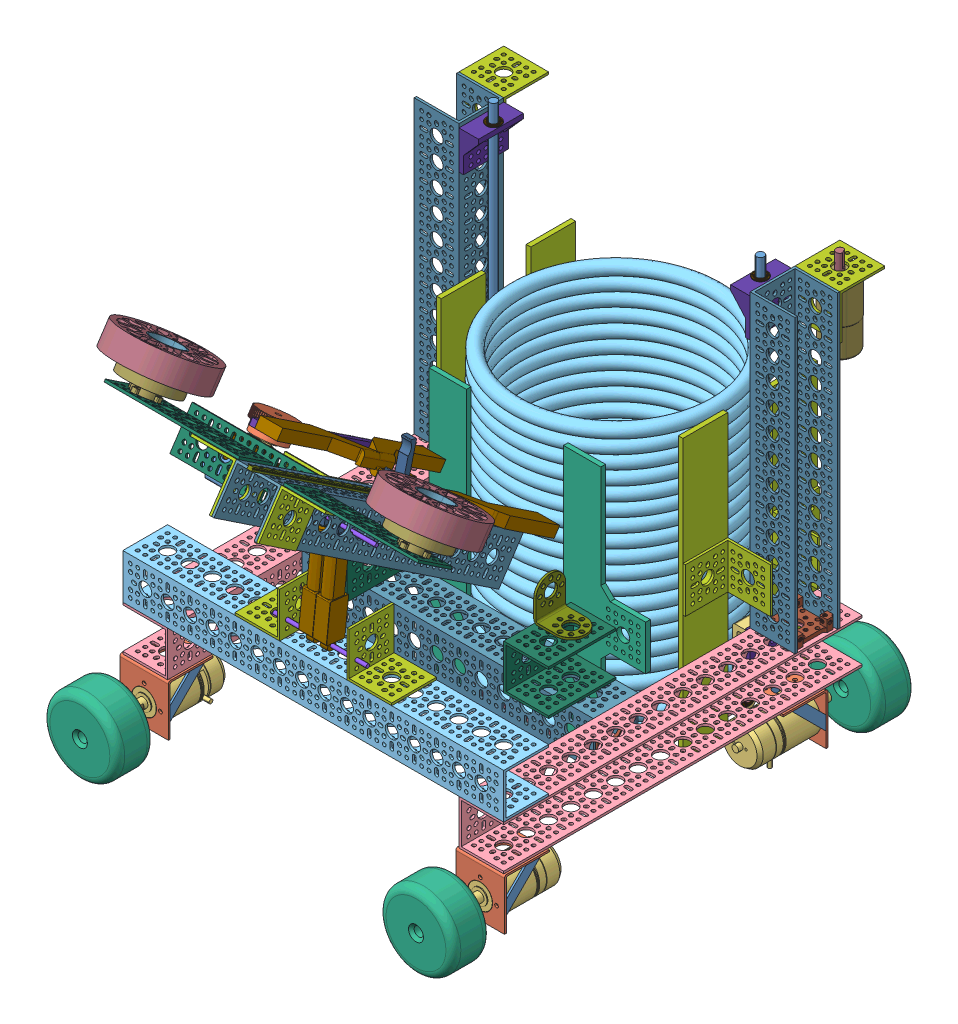
SolidWorks assembly 底座3.0, configuration 默认. Lengths in mm. (continued)
Mates (geometry in assembly coordinates): (continued)
- Concentric651: concentric anti-aligned: cylinder of 312mm-U型梁-7 through (105.3414 179.4201 525.5024) axis (0 1 0) radius 2; cone of 电机转向座-13 through (105.3414 186.9201 525.5024) axis (0 -1 0)
- Concentric652: concentric anti-aligned: cylinder of 312mm-U型梁-7 through (105.3414 181.4201 527.5024) axis (0 0 -1) radius 2; cone of 电机转向座-13 through (105.3414 181.4201 520.0024) axis (0 0 1)
- Concentric653: concentric anti-aligned: cylinder of 312mm-U型梁-7 through (105.3414 149.4201 527.5024) axis (0 0 -1) radius 2; cone of 电机转向座-13 through (105.3414 149.4201 520.0024) axis (0 0 1)
- Coincident318: coincident anti-aligned: plane of 384mm-U型梁-2 through (113.3414 189.4201 325.5024) normal (-1 0 0); plane of 电机转向座-13 through (113.3414 165.4201 541.5024) normal (1 0 0)
- Concentric654: concentric aligned: cylinder of 384mm-U型梁-2 through (123.3414 165.4201 541.5024) axis (-1 0 0) radius 7; cylinder of 电机转向座-13 through (113.3414 165.4201 541.5024) axis (-1 0 0) radius 7
- Concentric655: concentric aligned: cylinder of 384mm-U型梁-2 through (123.3414 156.9349 533.0171) axis (-1 0 0) radius 2; cylinder of 电机转向座-13 through (109.3414 156.9349 533.0171) axis (-1 0 0) radius 2
- Coincident323: coincident anti-aligned: plane of 312mm-U型梁-7 through (113.3414 189.4201 565.5024) normal (0 1 0); plane of 72mm-U型梁-5 through (89.3414 189.4201 589.5024) normal (0 -1 0)
- Coincident324: coincident anti-aligned: plane of 312mm-U型梁-7 through (113.3414 189.4201 565.5024) normal (0 1 0); plane of 72mm-U型梁-6 through (-174.6586 189.4201 589.5024) normal (0 -1 0)
- Concentric666: concentric aligned: cylinder of 72mm-U型梁-5 through (65.3414 227.4201 541.5024) axis (0 1 0) radius 7; cylinder of 圆角90°法兰-7 through (65.3414 237.4201 541.5024) axis (0 1 0) radius 7
- Coincident325: coincident anti-aligned: plane of 72mm-U型梁-5 through (89.3414 237.4201 589.5024) normal (0 1 0); plane of 圆角90°法兰-7 through (41.3414 237.4201 557.5024) normal (0 -1 0)
- Concentric667: concentric aligned: cylinder of 72mm-U型梁-5 through (54.0277 234.4201 541.5024) axis (0 1 0) radius 2; cylinder of 圆角90°法兰-7 through (54.0277 237.4201 541.5024) axis (0 1 0) radius 2.025
- Coincident326: coincident anti-aligned: plane of 72mm-U型梁-6 through (-174.6586 237.4201 589.5024) normal (0 1 0); plane of 圆角90°法兰-8 through (-126.6586 237.4201 525.5024) normal (0 -1 0)
- Concentric673: concentric anti-aligned: circle of 电动推杆2-1; cylinder of 升降轴-2 through (5.3414 358.1283 689.4197) axis (-1 0 0) radius 2
- Concentric674: concentric anti-aligned: circle of 电动推杆2-2; cylinder of 升降轴-2 through (5.3414 358.1283 689.4197) axis (-1 0 0) radius 2
- Coincident329: coincident anti-aligned: plane of 384mm-U型梁-1 through (-246.6586 189.4201 325.5024) normal (0 1 0); plane of 电机转向座-12 through (-222.6586 189.4201 373.5024) normal (0 -1 0)
- Concentric678: concentric aligned: cylinder of 轴承座-1 through (100.3414 497.4201 373.5024) axis (0 -1 0) radius 7; cylinder of 8-14轴承-7 through (100.3414 497.4201 373.5024) axis (0 -1 0) radius 7
- Coincident330: coincident anti-aligned: plane of 轴承座-1 through (113.3414 497.4201 397.5024) normal (0 1 0); plane of 8-14轴承-7 through (100.3414 497.4201 373.5024) normal (0 -1 0)
- Coincident331: coincident anti-aligned: plane of 384mm-U型梁-2 through (113.3414 189.4201 325.5024) normal (-1 0 0); plane of 轴承座-2 through (113.3414 145.4201 397.5024) normal (1 0 0)
- Concentric679: concentric anti-aligned: cylinder of 384mm-U型梁-2 through (123.3414 181.4201 389.5024) axis (-1 0 0) radius 2; cylinder of 轴承座-2 through (95.3414 181.4201 389.5024) axis (1 0 0) radius 2.05
- Concentric680: concentric anti-aligned: cylinder of 384mm-U型梁-2 through (123.3414 181.4201 357.5024) axis (-1 0 0) radius 2; cylinder of 轴承座-2 through (95.3414 181.4201 357.5024) axis (1 0 0) radius 2.05
- Concentric681: concentric anti-aligned: cylinder of 轴承座-2 through (100.3414 145.4201 373.5024) axis (0 1 0) radius 7; cylinder of 8-14轴承-8 through (100.3414 150.4201 373.5024) axis (0 -1 0) radius 7
- Coincident332: coincident anti-aligned: plane of 轴承座-2 through (113.3414 150.4201 349.5024) normal (0 1 0); plane of 8-14轴承-8 through (100.3414 150.4201 373.5024) normal (0 -1 0)
- Concentric682: concentric anti-aligned: cylinder of 8-14轴承-8 through (100.3414 146.4201 373.5024) axis (0 1 0) radius 4; cylinder of 螺纹杆-3 through (100.3414 517.4201 373.5024) axis (0 -1 0) radius 4
- Distance15: distance = 20 mm aligned: plane of 螺纹杆-3 through (100.3414 517.4201 373.5024) normal (0 1 0); plane of 轴承座-1 through (113.3414 497.4201 397.5024) normal (0 1 0)
- Concentric684: concentric aligned: cylinder of 螺纹杆-3 through (100.3414 517.4201 373.5024) axis (0 -1 0) radius 4; cylinder of 切边螺纹滑块-1 through (100.3414 178.1581 373.5024) axis (0 -1 0) radius 3.35
- Concentric687: concentric anti-aligned: cylinder of 384mm-U型梁-1 through (-208.6586 181.4201 389.5024) axis (1 0 0) radius 2; cylinder of 轴承座-4 through (-180.6586 181.4201 389.5024) axis (-1 0 0) radius 2.05
- Concentric688: concentric anti-aligned: cylinder of 384mm-U型梁-1 through (-208.6586 181.4201 357.5024) axis (1 0 0) radius 2; cylinder of 轴承座-4 through (-180.6586 181.4201 357.5024) axis (-1 0 0) radius 2.05
- Coincident334: coincident anti-aligned: plane of 384mm-U型梁-1 through (-198.6586 141.4201 325.5024) normal (1 0 0); plane of 轴承座-4 through (-198.6586 145.4201 349.5024) normal (-1 0 0)
- Concentric689: concentric aligned: cylinder of 轴承座-3 through (-185.6586 497.4201 373.5024) axis (0 -1 0) radius 7; cylinder of 8-14轴承-9 through (-185.6586 497.4201 373.5024) axis (0 -1 0) radius 7
- Coincident335: coincident anti-aligned: plane of 轴承座-3 through (-198.6586 497.4201 349.5024) normal (0 1 0); plane of 8-14轴承-9 through (-185.6586 497.4201 373.5024) normal (0 -1 0)
- Concentric690: concentric anti-aligned: cylinder of 轴承座-4 through (-185.6586 145.4201 373.5024) axis (0 1 0) radius 7; cylinder of 8-14轴承-10 through (-185.6586 150.4201 373.5024) axis (0 -1 0) radius 7
- Coincident336: coincident anti-aligned: plane of 轴承座-4 through (-198.6586 150.4201 397.5024) normal (0 1 0); plane of 8-14轴承-10 through (-185.6586 150.4201 373.5024) normal (0 -1 0)
- Concentric691: concentric anti-aligned: cylinder of 8-14轴承-9 through (-185.6586 493.4201 373.5024) axis (0 1 0) radius 4; cylinder of 螺纹杆-4 through (-185.6586 517.4201 373.5024) axis (0 -1 0) radius 4
- Coincident337: coincident aligned: plane of 螺纹杆-3 through (100.3414 517.4201 373.5024) normal (0 1 0); plane of 螺纹杆-4 through (-185.6586 517.4201 373.5024) normal (0 1 0)
- Concentric692: concentric aligned: cylinder of 螺纹杆-4 through (-185.6586 517.4201 373.5024) axis (0 -1 0) radius 4; cylinder of 切边螺纹滑块-2 through (-185.6586 178.1581 373.5024) axis (0 -1 0) radius 3.35
- Coincident338: coincident aligned: plane of 切边螺纹滑块-1 through (100.3414 168.1581 373.5024) normal (0 1 0); plane of 切边螺纹滑块-2 through (-185.6586 168.1581 373.5024) normal (0 1 0)
- Concentric693: concentric anti-aligned: cylinder of 切边螺纹滑块-1 through (100.3414 163.1581 373.5024) axis (0 1 0) radius 5.1; cylinder of 转换块-1 through (100.3414 173.1581 373.5024) axis (0 -1 0) radius 5.5
- Concentric694: concentric aligned: cylinder of 切边螺纹滑块-1 through (100.3414 168.1581 365.5024) axis (0 -1 0) radius 1.75; cylinder of 转换块-1 through (100.3414 173.1581 365.5024) axis (0 -1 0) radius 1.75
- Coincident339: coincident anti-aligned: plane of 切边螺纹滑块-1 through (100.3414 168.1581 373.5024) normal (0 1 0); plane of 转换块-1 through (100.3414 168.1581 373.5024) normal (0 -1 0)
- Concentric695: concentric anti-aligned: cylinder of 切边螺纹滑块-2 through (-185.6586 163.1581 373.5024) axis (0 1 0) radius 5.1; cylinder of 转换块-2 through (-185.6586 173.1581 373.5024) axis (0 -1 0) radius 5.5
- Concentric696: concentric aligned: cylinder of 切边螺纹滑块-2 through (-185.6586 168.1581 365.5024) axis (0 -1 0) radius 1.75; cylinder of 转换块-2 through (-185.6586 173.1581 365.5024) axis (0 -1 0) radius 1.75
- Coincident340: coincident anti-aligned: plane of 切边螺纹滑块-2 through (-185.6586 168.1581 373.5024) normal (0 1 0); plane of 转换块-2 through (-185.6586 168.1581 373.5024) normal (0 -1 0)
- Concentric697: concentric aligned: cylinder of 384mm-U型梁-2 through (121.3414 179.4201 365.5024) axis (0 1 0) radius 2; cylinder of 电机转向座-9 through (121.3414 193.4201 365.5024) axis (0 1 0) radius 2
- Concentric698: concentric anti-aligned: cone of 电机转向座-9 through (121.3414 197.4201 352.0024) axis (0 0 1); cylinder of 312mm-U型梁-8 through (121.3414 197.4201 359.5024) axis (0 0 -1) radius 2
- Concentric699: concentric anti-aligned: cone of 电机转向座-9 through (153.3414 197.4201 352.0024) axis (0 0 1); cylinder of 312mm-U型梁-8 through (153.3414 197.4201 359.5024) axis (0 0 -1) radius 2
- Concentric700: concentric anti-aligned: cone of 电机转向座-9 through (116.1914 197.4201 357.5024) axis (1 0 0); cylinder of 312mm-U型梁-8 through (123.3414 197.4201 357.5024) axis (-1 0 0) radius 2
- Concentric701: concentric anti-aligned: cone of 电机转向座-9 through (116.1914 197.4201 389.5024) axis (1 0 0); cylinder of 312mm-U型梁-8 through (123.3414 197.4201 389.5024) axis (-1 0 0) radius 2
- Coincident341: coincident anti-aligned: plane of 轴承座-1 through (113.3414 497.4201 349.5024) normal (1 0 0); plane of 312mm-U型梁-8 through (113.3414 189.4201 349.5024) normal (-1 0 0)
- Concentric704: concentric anti-aligned: cylinder of 48x48-L形支架-17 through (153.3414 493.4201 339.5024) axis (0 0 1) radius 2; cylinder of 312mm-U型梁-8 through (153.3414 493.4201 359.5024) axis (0 0 -1) radius 2
- Concentric705: concentric anti-aligned: cylinder of 48x48-L形支架-17 through (121.3414 493.4201 339.5024) axis (0 0 1) radius 2; cylinder of 312mm-U型梁-8 through (121.3414 493.4201 359.5024) axis (0 0 -1) radius 2
- Coincident342: coincident anti-aligned: plane of 48x48-L形支架-17 through (113.3414 501.4201 349.5024) normal (0 0 1); plane of 312mm-U型梁-8 through (161.3414 189.4201 349.5024) normal (0 0 -1)
- Concentric706: concentric anti-aligned: cylinder of 轴承座-1 through (95.3414 477.4201 357.5024) axis (1 0 0) radius 2.05; cylinder of 312mm-U型梁-8 through (123.3414 477.4201 357.5024) axis (-1 0 0) radius 2
- Concentric707: concentric anti-aligned: cylinder of 轴承座-1 through (95.3414 477.4201 389.5024) axis (1 0 0) radius 2.05; cylinder of 312mm-U型梁-8 through (123.3414 477.4201 389.5024) axis (-1 0 0) radius 2
- Concentric708: concentric aligned: cylinder of 384mm-U型梁-1 through (-206.6586 179.4201 365.5024) axis (0 1 0) radius 2; cylinder of 电机转向座-12 through (-206.6586 193.4201 365.5024) axis (0 1 0) radius 2
- Concentric709: concentric anti-aligned: cone of 电机转向座-12 through (-238.6586 197.4201 352.0024) axis (0 0 1); cylinder of 312mm-U型梁-9 through (-238.6586 197.4201 359.5024) axis (0 0 -1) radius 2
- Concentric710: concentric anti-aligned: cone of 电机转向座-12 through (-206.6586 197.4201 352.0024) axis (0 0 1); cylinder of 312mm-U型梁-9 through (-206.6586 197.4201 359.5024) axis (0 0 -1) radius 2
- Concentric711: concentric anti-aligned: cone of 电机转向座-12 through (-201.1586 197.4201 357.5024) axis (-1 0 0); cylinder of 312mm-U型梁-9 through (-208.6586 197.4201 357.5024) axis (1 0 0) radius 2
- Concentric712: concentric anti-aligned: cone of 电机转向座-12 through (-201.1586 197.4201 389.5024) axis (-1 0 0); cylinder of 312mm-U型梁-9 through (-208.6586 197.4201 389.5024) axis (1 0 0) radius 2
- Concentric713: concentric anti-aligned: cylinder of 48x48-L形支架-18 through (-206.6586 493.4201 339.5024) axis (0 0 1) radius 2; cylinder of 312mm-U型梁-9 through (-206.6586 493.4201 359.5024) axis (0 0 -1) radius 2
- Concentric714: concentric anti-aligned: cylinder of 48x48-L形支架-18 through (-238.6586 493.4201 339.5024) axis (0 0 1) radius 2; cylinder of 312mm-U型梁-9 through (-238.6586 493.4201 359.5024) axis (0 0 -1) radius 2
- Coincident343: coincident anti-aligned: plane of 48x48-L形支架-18 through (-246.6586 501.4201 349.5024) normal (0 0 1); plane of 312mm-U型梁-9 through (-246.6586 189.4201 349.5024) normal (0 0 -1)
- Concentric715: concentric anti-aligned: cylinder of 轴承座-3 through (-180.6586 477.4201 357.5024) axis (-1 0 0) radius 2.05; cylinder of 312mm-U型梁-9 through (-208.6586 477.4201 357.5024) axis (1 0 0) radius 2
- Concentric716: concentric anti-aligned: cylinder of 轴承座-3 through (-180.6586 477.4201 389.5024) axis (-1 0 0) radius 2.05; cylinder of 312mm-U型梁-9 through (-208.6586 477.4201 389.5024) axis (1 0 0) radius 2
- Coincident344: coincident anti-aligned: plane of 轴承座-3 through (-198.6586 497.4201 397.5024) normal (-1 0 0); plane of 312mm-U型梁-9 through (-198.6586 189.4201 397.5024) normal (1 0 0)
- Parallel5: parallel aligned: plane of 转换块-1 through (82.3414 173.1581 361.5024) normal (-1 0 0); plane of 312mm-U型梁-8 through (113.3414 189.4201 349.5024) normal (-1 0 0)
- Parallel6: parallel aligned: plane of 转换块-2 through (-167.6586 173.1581 385.5024) normal (1 0 0); plane of 312mm-U型梁-9 through (-198.6586 189.4201 397.5024) normal (1 0 0)
- Concentric717: concentric aligned: cylinder of 转换块-1 through (142.3414 100.1581 373.5024) axis (-1 0 0) radius 7; cylinder of 8-14轴承-11 through (87.3414 100.1581 373.5024) axis (-1 0 0) radius 7
- Coincident345: coincident anti-aligned: plane of 转换块-1 through (87.3414 88.1581 361.5024) normal (1 0 0); plane of 8-14轴承-11 through (87.3414 100.1581 373.5024) normal (-1 0 0)
- Concentric718: concentric aligned: cylinder of 转换块-2 through (-227.6586 100.1581 373.5024) axis (1 0 0) radius 7; cylinder of 8-14轴承-12 through (-172.6586 100.1581 373.5024) axis (1 0 0) radius 7
- Coincident346: coincident anti-aligned: plane of 转换块-2 through (-172.6586 88.1581 385.5024) normal (-1 0 0); plane of 8-14轴承-12 through (-172.6586 100.1581 373.5024) normal (1 0 0)
- Concentric719: concentric aligned: cylinder of 8-14轴承-11 through (83.3414 100.1581 373.5024) axis (1 0 0) radius 4; cylinder of 铲板-1 through (-164.6586 100.1581 373.5024) axis (1 0 0) radius 6
- Coincident347: coincident anti-aligned: plane of 8-14轴承-11 through (83.3414 100.1581 373.5024) normal (-1 0 0); plane of 铲板-1 through (83.3414 100.1581 373.5024) normal (1 0 0)
- Concentric720: concentric aligned: cylinder of 72mm-U型梁-6 through (-150.6586 227.4201 541.5024) axis (0 1 0) radius 7; cylinder of 圆角90°法兰-8 through (-150.6586 237.4201 541.5024) axis (0 1 0) radius 7
- Concentric728: concentric aligned: cylinder of 72mm-U型梁-6 through (-150.6586 234.4201 530.1887) axis (0 1 0) radius 2; cylinder of 圆角90°法兰-8 through (-150.6586 237.4201 530.1887) axis (0 1 0) radius 2.025
- Coincident356: coincident anti-aligned: plane of 312mm-U型梁-9 through (-246.6586 189.4201 397.5024) normal (0 0 1); plane of 48x48-L形支架-22 through (-174.6586 213.4201 397.5024) normal (0 0 -1)
- Concentric742: concentric anti-aligned: cylinder of 312mm-U型梁-9 through (-206.6586 253.4201 387.5024) axis (0 0 1) radius 2; cylinder of 48x48-L形支架-22 through (-206.6586 253.4201 407.5024) axis (0 0 -1) radius 2
- Concentric743: concentric anti-aligned: cylinder of 312mm-U型梁-9 through (-214.6586 253.4201 387.5024) axis (0 0 1) radius 2; cylinder of 48x48-L形支架-22 through (-214.6586 253.4201 407.5024) axis (0 0 -1) radius 2
- Coincident357: coincident anti-aligned: plane of 312mm-U型梁-9 through (-246.6586 189.4201 349.5024) normal (0 0 -1); plane of 48x48-L形支架-23 through (-174.6586 261.4201 349.5024) normal (0 0 1)
- Concentric744: concentric anti-aligned: cylinder of 312mm-U型梁-9 through (-206.6586 253.4201 359.5024) axis (0 0 -1) radius 2; cylinder of 48x48-L形支架-23 through (-206.6586 253.4201 339.5024) axis (0 0 1) radius 2
- Concentric745: concentric anti-aligned: cylinder of 312mm-U型梁-9 through (-214.6586 253.4201 359.5024) axis (0 0 -1) radius 2; cylinder of 48x48-L形支架-23 through (-214.6586 253.4201 339.5024) axis (0 0 1) radius 2
- Concentric746: concentric anti-aligned: cylinder of 48x48-L形支架-23 through (-184.6586 237.4201 325.5024) axis (1 0 0) radius 7; cylinder of 侧挡板-1 through (-169.6586 237.4201 325.5024) axis (-1 0 0) radius 7
- Coincident358: coincident anti-aligned: plane of 48x48-L形支架-23 through (-174.6586 261.4201 301.5024) normal (1 0 0); plane of 侧挡板-1 through (-174.6586 77.4201 301.5024) normal (-1 0 0)
- Concentric747: concentric anti-aligned: cylinder of 48x48-L形支架-23 through (-184.6586 253.4201 341.5024) axis (1 0 0) radius 2; cylinder of 侧挡板-1 through (-169.6586 253.4201 341.5024) axis (-1 0 0) radius 2
- Concentric748: concentric anti-aligned: cylinder of 48x48-L形支架-22 through (-184.6586 237.4201 421.5024) axis (1 0 0) radius 7; cylinder of 侧挡板-2 through (-169.6586 237.4201 421.5024) axis (-1 0 0) radius 7
- Concentric749: concentric anti-aligned: cylinder of 48x48-L形支架-22 through (-184.6586 253.4201 437.5024) axis (1 0 0) radius 2; cylinder of 侧挡板-2 through (-169.6586 253.4201 437.5024) axis (-1 0 0) radius 2
- Coincident359: coincident anti-aligned: plane of 48x48-L形支架-22 through (-174.6586 213.4201 445.5024) normal (1 0 0); plane of 侧挡板-2 through (-174.6586 77.4201 397.5024) normal (-1 0 0)
- Coincident360: coincident anti-aligned: plane of 312mm-U型梁-8 through (161.3414 189.4201 349.5024) normal (0 0 -1); plane of 48x48-L形支架-24 through (137.3414 261.4201 349.5024) normal (0 0 1)
- Concentric750: concentric anti-aligned: cylinder of 312mm-U型梁-8 through (121.3414 253.4201 359.5024) axis (0 0 -1) radius 2; cylinder of 48x48-L形支架-24 through (121.3414 253.4201 339.5024) axis (0 0 1) radius 2
- Concentric751: concentric anti-aligned: cylinder of 312mm-U型梁-8 through (129.3414 253.4201 359.5024) axis (0 0 -1) radius 2; cylinder of 48x48-L形支架-24 through (129.3414 253.4201 339.5024) axis (0 0 1) radius 2
- Concentric752: concentric aligned: cylinder of 侧挡板-3 through (89.3414 237.4201 325.5024) axis (-1 0 0) radius 7; cylinder of 48x48-L形支架-24 through (99.3414 237.4201 325.5024) axis (-1 0 0) radius 7
- Coincident361: coincident anti-aligned: plane of 侧挡板-3 through (89.3414 77.4201 301.5024) normal (1 0 0); plane of 48x48-L形支架-24 through (89.3414 261.4201 349.5024) normal (-1 0 0)
- Concentric753: concentric aligned: cylinder of 侧挡板-3 through (89.3414 253.4201 309.5024) axis (-1 0 0) radius 2; cylinder of 48x48-L形支架-24 through (99.3414 253.4201 309.5024) axis (-1 0 0) radius 2
- Coincident362: coincident anti-aligned: plane of 312mm-U型梁-8 through (161.3414 189.4201 397.5024) normal (0 0 1); plane of 48x48-L形支架-25 through (89.3414 261.4201 397.5024) normal (0 0 -1)
- Concentric754: concentric anti-aligned: cylinder of 312mm-U型梁-8 through (121.3414 253.4201 387.5024) axis (0 0 1) radius 2; cylinder of 48x48-L形支架-25 through (121.3414 253.4201 407.5024) axis (0 0 -1) radius 2
- Concentric755: concentric anti-aligned: cylinder of 312mm-U型梁-8 through (129.3414 253.4201 387.5024) axis (0 0 1) radius 2; cylinder of 48x48-L形支架-25 through (129.3414 253.4201 407.5024) axis (0 0 -1) radius 2
- Concentric756: concentric aligned: cylinder of 侧挡板-4 through (89.3414 237.4201 421.5024) axis (-1 0 0) radius 7; cylinder of 48x48-L形支架-25 through (99.3414 237.4201 421.5024) axis (-1 0 0) radius 7
- Coincident363: coincident anti-aligned: plane of 侧挡板-4 through (89.3414 77.4201 397.5024) normal (1 0 0); plane of 48x48-L形支架-25 through (89.3414 261.4201 445.5024) normal (-1 0 0)
- Concentric757: concentric aligned: cylinder of 侧挡板-4 through (89.3414 253.4201 437.5024) axis (-1 0 0) radius 2; cylinder of 48x48-L形支架-25 through (99.3414 253.4201 437.5024) axis (-1 0 0) radius 2
- 同心2: concentric aligned: circle of 圆角90°法兰-8; circle of 312mm-U型梁-10
- 距离2: distance = 60 mm anti-aligned: plane of 312mm-U型梁-10 through (-66.6586 401.3085 794.3883) normal (-1 0 0); plane of 圆角90°法兰-8 through (-126.6586 237.4201 525.5024) normal (1 0 0)
- 同心9: concentric anti-aligned: circle of 312mm-U型梁-10; circle of 滑轨9-1
- 重合17: coincident anti-aligned: plane of 312mm-U型梁-10 through (-66.6586 441.2359 767.7462) normal (0 0.831822 -0.555042); plane of 滑轨9-1 through (-40.1586 271.5672 513.4695) normal (0 -0.831822 0.555042)
- 平行4: parallel aligned: plane of 312mm-U型梁-10 through (-21.1586 439.1564 769.1339) normal (-1 0 0); plane of 滑轨9-1 through (-45.1586 271.5672 513.4695) normal (-1 0 0)
- 重合19: coincident anti-aligned: plane of 蜘蛛钩子-1/滑块1-1 through (-40.1586 335.1761 602.1319) normal (0 -0.831822 0.555042); plane of 滑轨9-1 through (-45.1586 274.645 511.4159) normal (0 0.831822 -0.555042)
- 重合20: coincident: line of 蜘蛛钩子-1/滑块1-1 through (-44.6586 342.8091 616.2736) axis (-0.707107 -0.588187 0.392474); plane of 滑轨9-1 through (-44.6586 273.3972 512.2485) normal (-0.707107 0.588187 -0.392474)
- 重合21: coincident anti-aligned: plane of 蜘蛛钩子-1/滑块座1-1 through (-115.6586 311.2353 689.2916) normal (-1 0 0); plane of 齿条(1)-1 through (-115.6586 355.6063 610.1389) normal (1 0 0)
- 重合22: coincident aligned: plane of 蜘蛛钩子-1/滑块座1-1 through (-97.6586 375.7779 646.2249) normal (0 -0.831822 0.555042); plane of 齿条(1)-1 through (-123.1586 289.073 516.2832) normal (0 -0.831822 0.555042)
- 重合23: coincident aligned: plane of 蜘蛛钩子-1/滑块座1-1 through (-115.6586 403.6958 704.2795) normal (0 0.555042 0.831822); plane of 齿条(1)-1 through (-115.6586 408.2709 701.2268) normal (0 0.555042 0.831822)
- 重合30: coincident anti-aligned: plane of 齿轮(5.23)-1 through (-143.7715 366.6942 656.9339) normal (0 -0.831822 0.555042); plane of 舵盘(5.23-1 through (-143.7715 366.6942 656.9339) normal (0 0.831822 -0.555042)
- 重合31: coincident aligned: plane of 齿条(1)-1 through (-123.1586 294.4799 512.6754) normal (0 0.831822 -0.555042); plane of 齿轮(5.23)-1 through (-143.7715 383.3306 645.833) normal (0 0.831822 -0.555042)
- 同心16: concentric anti-aligned: circle of 312mm-U型梁-10; circle of 48x48-L形支架-27
- 重合34: coincident anti-aligned: plane of 312mm-U型梁-10 through (-66.6586 401.3085 794.3883) normal (-1 0 0); plane of 48x48-L形支架-27 through (-66.6586 347.9889 628.0001) normal (1 0 0)
- 同心17: concentric anti-aligned: cylinder of 312mm-U型梁-7 through (-166.6586 179.4201 557.5024) axis (0 1 0) radius 2; circle of 72mm-U型梁-6
- 同心19: concentric anti-aligned: circle of 312mm-U型梁-7; circle of 72mm-U型梁-5
- 同心20: concentric anti-aligned: circle of 圆角90°法兰-7; circle of 312mm-U型梁-10
- 同心5: concentric anti-aligned: circle of 发射法兰1-1; circle of 发射无刷电机-1
- 重合4: coincident anti-aligned: circle of 发射法兰1-1; plane of 发射无刷电机-1 through (-186.6586 458.3921 738.8671) normal (0 0.831822 -0.555042)
- 同心21: concentric anti-aligned: circle of 发射法兰1-1; circle of 摩擦轮-1/摩擦轮.STEP-1/3613-0014-0096 Core.STEP-1
- 重合5: coincident anti-aligned: plane of 发射法兰1-1 through (-186.6586 457.2783 728.1895) normal (0 0.831822 -0.555042); plane of 摩擦轮-1/摩擦轮.STEP-1/3613-0014-0096 Core.STEP-1 through (-186.6586 457.2783 728.1895) normal (0 -0.831822 0.555042)
- 同心22: concentric anti-aligned: circle of 发射无刷电机-1; circle of 5孔平板-1
- 重合3: coincident anti-aligned: plane of 发射无刷电机-1 through (-186.6586 429.9945 746.3949) normal (0 -0.831822 0.555042); plane of 5孔平板-1 through (-66.6586 418.0611 728.5107) normal (0 0.831822 -0.555042)
- 同心1: concentric aligned: unknown of 5孔平板-1; unknown of 48x48-L形支架-28
- 平行1: parallel aligned: plane of 5孔平板-1 through (-210.6586 435.9453 716.5773) normal (-1 0 0); plane of 48x48-L形支架-28 through (-114.6586 439.1564 769.1339) normal (-1 0 0)
- 同心23: concentric anti-aligned: circle of 312mm-U型梁-10; circle of 48x48-L形支架-28
- 重合35: coincident aligned: plane of 312mm-U型梁-10 through (-42.6586 439.1564 769.1339) normal (0 0.555042 0.831822); plane of 48x48-L形支架-28 through (-69.1586 421.2722 781.0673) normal (0 0.555042 0.831822)
- 重合36: coincident anti-aligned: plane of 312mm-U型梁-10 through (-66.6586 401.3085 794.3883) normal (-1 0 0); plane of 48x48-L形支架-28 through (-66.6586 441.2359 767.7462) normal (1 0 0)
- 同心24: concentric anti-aligned: circle of 发射法兰1-2; circle of 发射无刷电机-2
- 重合37: coincident anti-aligned: circle of 发射法兰1-2; plane of 发射无刷电机-2 through (101.3414 447.8463 723.0624) normal (0 0.831822 -0.555042)
- 同心6: concentric anti-aligned: circle of 发射法兰1-2; circle of 摩擦轮-2/摩擦轮.STEP-1/3613-0014-0096 Core.STEP-1
- 重合38: coincident anti-aligned: plane of 发射法兰1-2 through (101.3414 457.2783 728.1895) normal (0 0.831822 -0.555042); plane of 摩擦轮-2/摩擦轮.STEP-1/3613-0014-0096 Core.STEP-1 through (101.3414 457.2783 728.1895) normal (0 -0.831822 0.555042)
- 同心25: concentric anti-aligned: circle of 发射无刷电机-2; circle of 5孔平板-2
- 重合39: coincident anti-aligned: plane of 发射无刷电机-2 through (101.3414 429.9945 746.3949) normal (0 -0.831822 0.555042); plane of 5孔平板-2 through (-18.6586 441.9279 764.2791) normal (0 0.831822 -0.555042)
- 同心26: concentric aligned: unknown of 5孔平板-2; unknown of 48x48-L形支架-29
- 平行8: parallel aligned: plane of 5孔平板-2 through (125.3414 459.8121 752.3457) normal (1 0 0); plane of 48x48-L形支架-29 through (29.3414 412.5144 729.2064) normal (1 0 0)
- 同心27: concentric aligned: circle of 312mm-U型梁-10; circle of 48x48-L形支架-29
- 重合40: coincident aligned: plane of 312mm-U型梁-10 through (-42.6586 439.1564 769.1339) normal (0 0.555042 0.831822); plane of 48x48-L形支架-29 through (-16.1586 421.2722 781.0673) normal (0 0.555042 0.831822)
- 重合41: coincident anti-aligned: plane of 312mm-U型梁-10 through (-18.6586 401.3085 794.3883) normal (1 0 0); plane of 48x48-L形支架-29 through (-18.6586 414.5939 727.8188) normal (-1 0 0)
- 同心28: concentric aligned: circle of 舵机-1; circle of 多功能舵机支架(1)-1
- 重合2: coincident anti-aligned: plane of 舵机-1 through (-179.2715 356.9383 673.6621) normal (0 -0.831822 0.555042); plane of 多功能舵机支架(1)-1 through (-153.6215 359.7413 677.8628) normal (0 0.831822 -0.555042)
- 同心29: concentric anti-aligned: circle of 舵机-1; circle of 齿轮(5.23)-1
- 同心30: concentric anti-aligned: circle of 舵机-1; circle of 舵盘(5.23-1
- 重合42: coincident anti-aligned: plane of 舵机-1 through (-143.7715 362.951 659.4316) normal (0 0.831822 -0.555042); plane of 舵盘(5.23-1 through (-143.7715 362.951 659.4316) normal (0 -0.831822 0.555042)
- 平行9: parallel aligned: plane of 48x48-L形支架-28 through (-69.1586 421.2722 781.0673) normal (0 0.555042 0.831822); plane of 多功能舵机支架(1)-1 through (-182.6215 359.7413 677.8628) normal (0 0.555042 0.831822)
- 平行12: parallel anti-aligned: plane of 舵机-1 through (-179.2715 360.0168 673.4112) normal (0 0.555042 0.831822); plane of 多功能舵机支架(1)-1 through (-174.1215 332.4288 693.683) normal (0 -0.555042 -0.831822)
- 重合53: coincident anti-aligned: plane of 5孔平板-1 through (-66.6586 441.2359 767.7462) normal (0 -0.831822 0.555042); plane of 48x48-L形支架-28 through (-114.6586 441.2359 767.7462) normal (0 0.831822 -0.555042)
- 重合54: coincident anti-aligned: plane of 5孔平板-2 through (-18.6586 414.5939 727.8188) normal (0 -0.831822 0.555042); plane of 48x48-L形支架-29 through (29.3414 414.5939 727.8188) normal (0 0.831822 -0.555042)
- 平行13: parallel aligned: plane of 312mm-U型梁-10 through (-42.6586 439.1564 769.1339) normal (0 0.555042 0.831822); plane of 48x48-L形支架-27 through (-66.6586 374.6309 667.9276) normal (0 0.555042 0.831822)
- 同心38: concentric aligned: circle of 48x48-L形支架-27; circle of 5孔平板-3
- 重合57: coincident anti-aligned: plane of 48x48-L形支架-27 through (-66.6586 374.6309 667.9276) normal (0 0.555042 0.831822); plane of 5孔平板-3 through (-66.6586 334.7034 694.5696) normal (0 -0.555042 -0.831822)
- 重合58: coincident anti-aligned: plane of 多功能舵机支架(1)-1 through (-182.6215 359.7413 677.8628) normal (0 0.555042 0.831822); plane of 5孔平板-3 through (-66.6586 334.7034 694.5696) normal (0 -0.555042 -0.831822)
